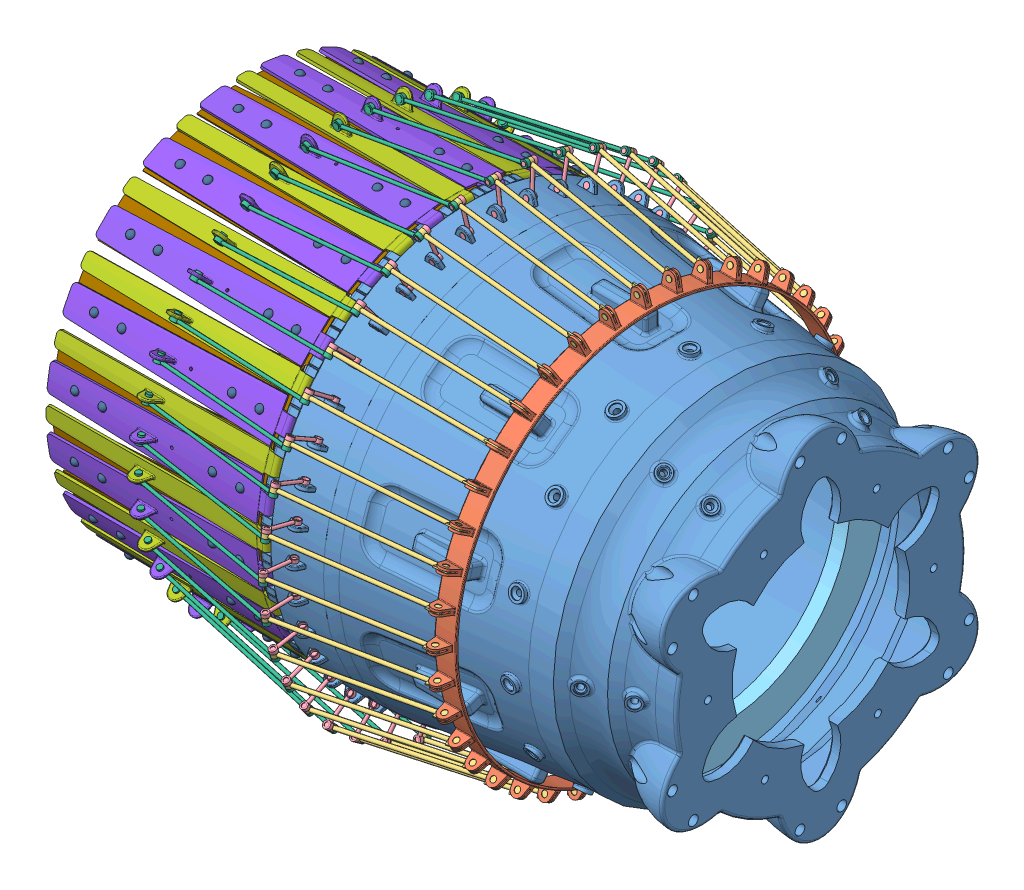
SolidWorks assembly Exhaust Assembly, configuration OPEN . Lengths in mm.
Overall size (418.47 373.17 373.17).
263 component instances, 10 part files, 37 mates.
Components (placement in the parent):
- Part1-1: Part1 [Default] at (233.2329 170.9628 321.4261) size (260.63 300.09 300.09)
- Flare Base-1: Flare Base [Default] at (-84.7671 170.9628 321.4261) x (0 -0.156434 -0.987688) z (1 0 0) size (303.2 303.2 15)
- Flare lever 2-1: Flare lever 2 [Default] at (-182.2053 335.9675 321.4261) x (0 0 -1) z (0.985354 -0.170521 0) size (4.1 7 113)
- Flare Lever 3-1: Flare Lever 3 [Default] at (-182.008 318.4395 318.6761) x (0 0 1) z (-0.120444 0.99272 0) size (8.2 5 25)
- Heat Ring-1: Heat Ring [Default] at (-17.9374 170.9628 321.4261) x (0 -0.257651 0.966238) z (-1 0 0) size (230 230 10)
- Flare Lever 3-2: Flare Lever 3 [Default] at (-182.008 316.1937 295.6395) x (0 0.156434 0.987688) z (-0.120444 0.980498 -0.155296) size (8.2 5 25)
- Flare lever 2-2: Flare lever 2 [Default] at (-182.2053 333.936 295.6137) x (0 -0.156434 -0.987688) z (0.985354 -0.168421 0.026675) size (4.1 7 113)
- Flare lever 1-3: Flare lever 1 [Default] at (-237.8374 326.7848 324.1761) x (0 0 1) z (-0.984613 -0.174748 0) size (6.1 6 116)
- Blade 3-4: Blade 3 [Default] at (-266.5909 130.4236 321.4261) x (0.957917 -0.287045 0) z (0 0 1) size (154.82 49.98 15.19)
- Flare lever 1-4: Flare lever 1 [Default] at (-237.8374 325.2965 299.7663) x (0 0.156434 0.987688) z (-0.984613 -0.172596 0.027337) size (6.1 6 116)
- Blade 4-1: Blade 4 [Default] at (-253.5304 173.9713 320.9496) x (0.957917 -0.283511 0.044904) z (0 0.156434 0.987688) size (154.82 50.19 28.4)
- Blade 1-2: Blade 1 [Default] at (-254.9478 304.5579 299.0391) x (0.957809 -0.285754 0.030748) z (0.017578 0.165029 0.986132) size (146.12 48.38 42.15)
- Rivet-1: Rivet [Default] at (-225.6117 310.4186 298.8323) x (0.988427 0.034217 0.147786) z (0.15131 -0.153019 -0.976571) size (5.66 11 5.66)
- Rivet-2: Rivet [Default] at (-245.6106 310.2053 298.866) x (0.133203 0.156461 0.978661) z (0.99103 -0.010266 -0.133245) size (5.66 11 5.66)
- Rivet-3: Rivet [Default] at (-325.6059 309.3518 299.0012) x (0.133203 0.156461 0.978661) z (0.99103 -0.010266 -0.133245) size (5.66 11 5.66)
- Rivet-4: Rivet [Default] at (-345.6047 309.1385 299.035) x (0.241866 0.15437 0.957951) z (0.97025 -0.027487 -0.240541) size (5.66 11 5.66)
- Rivet-5: Rivet [Default] at (-345.6047 309.2949 342.8295) x (0.241866 -0.149209 0.958769) z (0.97025 0.04819 -0.237263) size (5.66 11 5.66)
- Rivet-6: Rivet [Default] at (-345.6047 295.9104 384.5289) x (0.241866 -0.438182 0.865735) z (0.97025 0.119149 -0.210759) size (5.66 11 5.66)
- Rivet-7: Rivet [Default] at (-345.6047 270.2952 420.0514) x (0.241866 -0.684263 0.687957) z (0.97025 0.178446 -0.163624) size (5.66 11 5.66)
- Rivet-8: Rivet [Default] at (-345.6047 234.9566 445.9198) x (0.241866 -0.863363 0.442838) z (0.97025 0.220275 -0.100473) size (5.66 11 5.66)
- Rivet-9: Rivet [Default] at (-345.6047 193.3539 459.6018) x (0.241866 -0.957951 0.15437) z (0.97025 0.240541 -0.027487) size (5.66 11 5.66)
- Rivet-10: Rivet [Default] at (-345.6047 149.5594 459.7582) x (0.241866 -0.958769 -0.149209) z (0.97025 0.237263 0.04819) size (5.66 11 5.66)
- Rivet-11: Rivet [Default] at (-345.6047 107.86 446.3737) x (0.241866 -0.865735 -0.438182) z (0.97025 0.210759 0.119149) size (5.66 11 5.66)
- Rivet-12: Rivet [Default] at (-345.6047 72.3375 420.7585) x (0.241866 -0.687957 -0.684263) z (0.97025 0.163624 0.178446) size (5.66 11 5.66)
- Rivet-13: Rivet [Default] at (-345.6047 46.4692 385.42) x (0.241866 -0.442838 -0.863363) z (0.97025 0.100473 0.220275) size (5.66 11 5.66)
- Rivet-14: Rivet [Default] at (-345.6047 32.7871 343.8172) x (0.241866 -0.15437 -0.957951) z (0.97025 0.027487 0.240541) size (5.66 11 5.66)
- Rivet-15: Rivet [Default] at (-345.6047 32.6307 300.0227) x (0.241866 0.149209 -0.958769) z (0.97025 -0.04819 0.237263) size (5.66 11 5.66)
- Rivet-16: Rivet [Default] at (-345.6047 46.0152 258.3233) x (0.241866 0.438182 -0.865735) z (0.97025 -0.119149 0.210759) size (5.66 11 5.66)
- Rivet-17: Rivet [Default] at (-345.6047 71.6304 222.8008) x (0.241866 0.684263 -0.687957) z (0.97025 -0.178446 0.163624) size (5.66 11 5.66)
- Rivet-18: Rivet [Default] at (-345.6047 106.969 196.9325) x (0.241866 0.863363 -0.442838) z (0.97025 -0.220275 0.100473) size (5.66 11 5.66)
- Rivet-19: Rivet [Default] at (-345.6047 148.5717 183.2505) x (0.241866 0.957951 -0.15437) z (0.97025 -0.240541 0.027487) size (5.66 11 5.66)
- Rivet-20: Rivet [Default] at (-345.6047 192.3662 183.094) x (0.241866 0.958769 0.149209) z (0.97025 -0.237263 -0.04819) size (5.66 11 5.66)
- Rivet-21: Rivet [Default] at (-345.6047 234.0656 196.4785) x (0.241866 0.865735 0.438182) z (0.97025 -0.210759 -0.119149) size (5.66 11 5.66)
- Rivet-22: Rivet [Default] at (-345.6047 269.5881 222.0937) x (0.241866 0.687957 0.684263) z (0.97025 -0.163624 -0.178446) size (5.66 11 5.66)
- Rivet-23: Rivet [Default] at (-345.6047 295.4564 257.4323) x (0.241866 0.442838 0.863363) z (0.97025 -0.100473 -0.220275) size (5.66 11 5.66)
- Rivet-24: Rivet [Default] at (-325.6059 309.5083 342.8633) x (0.133203 -0.153619 0.979111) z (0.99103 0.031412 -0.129896) size (5.66 11 5.66)
- Rivet-25: Rivet [Default] at (-325.6059 296.1029 384.627) x (0.133203 -0.448662 0.883719) z (0.99103 0.070014 -0.113832) size (5.66 11 5.66)
- Rivet-26: Rivet [Default] at (-325.6059 270.4479 420.2042) x (0.133203 -0.699787 0.701822) z (0.99103 0.101764 -0.086625) size (5.66 11 5.66)
- Rivet-27: Rivet [Default] at (-325.6059 235.0547 446.1122) x (0.133203 -0.882412 0.451226) z (0.99103 0.123552 -0.050939) size (5.66 11 5.66)
- Rivet-28: Rivet [Default] at (-325.6059 193.3877 459.8151) x (0.133203 -0.978661 0.156461) z (0.99103 0.133245 -0.010266) size (5.66 11 5.66)
- Rivet-29: Rivet [Default] at (-325.6059 149.5256 459.9716) x (0.133203 -0.979111 -0.153619) z (0.99103 0.129896 0.031412) size (5.66 11 5.66)
- Rivet-30: Rivet [Default] at (-325.6059 107.7619 446.5662) x (0.133203 -0.883719 -0.448662) z (0.99103 0.113832 0.070014) size (5.66 11 5.66)
- Rivet-31: Rivet [Default] at (-325.6059 72.1847 420.9113) x (0.133203 -0.701822 -0.699787) z (0.99103 0.086625 0.101764) size (5.66 11 5.66)
- Rivet-32: Rivet [Default] at (-325.6059 46.2767 385.518) x (0.133203 -0.451226 -0.882412) z (0.99103 0.050939 0.123552) size (5.66 11 5.66)
- Rivet-33: Rivet [Default] at (-325.6059 32.5738 343.851) x (0.133203 -0.156461 -0.978661) z (0.99103 0.010266 0.133245) size (5.66 11 5.66)
- Rivet-34: Rivet [Default] at (-325.6059 32.4173 299.9889) x (0.133203 0.153619 -0.979111) z (0.99103 -0.031412 0.129896) size (5.66 11 5.66)
- Rivet-35: Rivet [Default] at (-325.6059 45.8227 258.2252) x (0.133203 0.448662 -0.883719) z (0.99103 -0.070014 0.113832) size (5.66 11 5.66)
- Rivet-36: Rivet [Default] at (-325.6059 71.4776 222.6481) x (0.133203 0.699787 -0.701822) z (0.99103 -0.101764 0.086625) size (5.66 11 5.66)
- Rivet-37: Rivet [Default] at (-325.6059 106.8709 196.74) x (0.133203 0.882412 -0.451226) z (0.99103 -0.123552 0.050939) size (5.66 11 5.66)
- Rivet-38: Rivet [Default] at (-325.6059 148.5379 183.0371) x (0.133203 0.978661 -0.156461) z (0.99103 -0.133245 0.010266) size (5.66 11 5.66)
- Rivet-39: Rivet [Default] at (-325.6059 192.4 182.8807) x (0.133203 0.979111 0.153619) z (0.99103 -0.129896 -0.031412) size (5.66 11 5.66)
- Rivet-40: Rivet [Default] at (-325.6059 234.1637 196.286) x (0.133203 0.883719 0.448662) z (0.99103 -0.113832 -0.070014) size (5.66 11 5.66)
- Rivet-41: Rivet [Default] at (-325.6059 269.7408 221.941) x (0.133203 0.701822 0.699787) z (0.99103 -0.086625 -0.101764) size (5.66 11 5.66)
- Rivet-42: Rivet [Default] at (-325.6059 295.6489 257.3342) x (0.133203 0.451226 0.882412) z (0.99103 -0.050939 -0.123552) size (5.66 11 5.66)
- Rivet-43: Rivet [Default] at (-245.6106 310.3617 342.9985) x (0.133203 -0.153619 0.979111) z (0.99103 0.031412 -0.129896) size (5.66 11 5.66)
- Rivet-44: Rivet [Default] at (-245.6106 296.8728 385.0193) x (0.133203 -0.448662 0.883719) z (0.99103 0.070014 -0.113832) size (5.66 11 5.66)
- Rivet-45: Rivet [Default] at (-245.6106 271.0589 420.8152) x (0.133203 -0.699787 0.701822) z (0.99103 0.101764 -0.086625) size (5.66 11 5.66)
- Rivet-46: Rivet [Default] at (-245.6106 235.447 446.8821) x (0.133203 -0.882412 0.451226) z (0.99103 0.123552 -0.050939) size (5.66 11 5.66)
- Rivet-47: Rivet [Default] at (-245.6106 193.5229 460.6686) x (0.133203 -0.978661 0.156461) z (0.99103 0.133245 -0.010266) size (5.66 11 5.66)
- Rivet-48: Rivet [Default] at (-245.6106 149.3904 460.825) x (0.133203 -0.979111 -0.153619) z (0.99103 0.129896 0.031412) size (5.66 11 5.66)
- Rivet-49: Rivet [Default] at (-245.6106 107.3696 447.3361) x (0.133203 -0.883719 -0.448662) z (0.99103 0.113832 0.070014) size (5.66 11 5.66)
- Rivet-50: Rivet [Default] at (-245.6106 71.5738 421.5223) x (0.133203 -0.701822 -0.699787) z (0.99103 0.086625 0.101764) size (5.66 11 5.66)
- Rivet-51: Rivet [Default] at (-245.6106 45.5068 385.9103) x (0.133203 -0.451226 -0.882412) z (0.99103 0.050939 0.123552) size (5.66 11 5.66)
- Rivet-52: Rivet [Default] at (-245.6106 31.7203 343.9862) x (0.133203 -0.156461 -0.978661) z (0.99103 0.010266 0.133245) size (5.66 11 5.66)
- Rivet-53: Rivet [Default] at (-245.6106 31.5639 299.8537) x (0.133203 0.153619 -0.979111) z (0.99103 -0.031412 0.129896) size (5.66 11 5.66)
- Rivet-54: Rivet [Default] at (-245.6106 45.0528 257.8329) x (0.133203 0.448662 -0.883719) z (0.99103 -0.070014 0.113832) size (5.66 11 5.66)
- Rivet-55: Rivet [Default] at (-245.6106 70.8666 222.0371) x (0.133203 0.699787 -0.701822) z (0.99103 -0.101764 0.086625) size (5.66 11 5.66)
- Rivet-56: Rivet [Default] at (-245.6106 106.4786 195.9701) x (0.133203 0.882412 -0.451226) z (0.99103 -0.123552 0.050939) size (5.66 11 5.66)
- Rivet-57: Rivet [Default] at (-245.6106 148.4027 182.1837) x (0.133203 0.978661 -0.156461) z (0.99103 -0.133245 0.010266) size (5.66 11 5.66)
- Rivet-58: Rivet [Default] at (-245.6106 192.5352 182.0272) x (0.133203 0.979111 0.153619) z (0.99103 -0.129896 -0.031412) size (5.66 11 5.66)
- Rivet-59: Rivet [Default] at (-245.6106 234.556 195.5161) x (0.133203 0.883719 0.448662) z (0.99103 -0.113832 -0.070014) size (5.66 11 5.66)
- Rivet-60: Rivet [Default] at (-245.6106 270.3518 221.33) x (0.133203 0.701822 0.699787) z (0.99103 -0.086625 -0.101764) size (5.66 11 5.66)
- Rivet-61: Rivet [Default] at (-245.6106 296.4188 256.9419) x (0.133203 0.451226 0.882412) z (0.99103 -0.050939 -0.123552) size (5.66 11 5.66)
- Rivet-62: Rivet [Default] at (-225.6117 310.5751 343.0323) x (0.988427 -0.013126 0.151126) z (0.15131 0.156247 -0.976059) size (5.66 11 5.66)
- Rivet-63: Rivet [Default] at (-225.6117 297.0653 385.1174) x (0.988427 -0.059184 0.139673) z (0.15131 0.450219 -0.880005) size (5.66 11 5.66)
- Rivet-64: Rivet [Default] at (-225.6117 271.2117 420.9679) x (0.988427 -0.099449 0.114548) z (0.15131 0.70012 -0.697809) size (5.66 11 5.66)
- Rivet-65: Rivet [Default] at (-225.6117 235.5451 447.0746) x (0.988427 -0.129979 0.07821) z (0.15131 0.881489 -0.447307) size (5.66 11 5.66)
- Rivet-66: Rivet [Default] at (-225.6117 193.5567 460.8819) x (0.988427 -0.147786 0.034217) z (0.15131 0.976571 -0.153019) size (5.66 11 5.66)
- Rivet-67: Rivet [Default] at (-225.6117 149.3566 461.0384) x (0.988427 -0.151126 -0.013126) z (0.15131 0.976059 0.156247) size (5.66 11 5.66)
- Rivet-68: Rivet [Default] at (-225.6117 107.2715 447.5286) x (0.988427 -0.139673 -0.059184) z (0.15131 0.880005 0.450219) size (5.66 11 5.66)
- Rivet-69: Rivet [Default] at (-225.6117 71.421 421.675) x (0.988427 -0.114548 -0.099449) z (0.15131 0.697809 0.70012) size (5.66 11 5.66)
- Rivet-70: Rivet [Default] at (-225.6117 45.3143 386.0084) x (0.988427 -0.07821 -0.129979) z (0.15131 0.447307 0.881489) size (5.66 11 5.66)
- Rivet-71: Rivet [Default] at (-225.6117 31.507 344.02) x (0.988427 -0.034217 -0.147786) z (0.15131 0.153019 0.976571) size (5.66 11 5.66)
- Rivet-72: Rivet [Default] at (-225.6117 31.3505 299.8199) x (0.988427 0.013126 -0.151126) z (0.15131 -0.156247 0.976059) size (5.66 11 5.66)
- Rivet-73: Rivet [Default] at (-225.6117 44.8603 257.7349) x (0.988427 0.059184 -0.139673) z (0.15131 -0.450219 0.880005) size (5.66 11 5.66)
- Rivet-74: Rivet [Default] at (-225.6117 70.7139 221.8843) x (0.988427 0.099449 -0.114548) z (0.15131 -0.70012 0.697809) size (5.66 11 5.66)
- Rivet-75: Rivet [Default] at (-225.6117 106.3805 195.7776) x (0.988427 0.129979 -0.07821) z (0.15131 -0.881489 0.447307) size (5.66 11 5.66)
- Rivet-76: Rivet [Default] at (-225.6117 148.3689 181.9703) x (0.988427 0.147786 -0.034217) z (0.15131 -0.976571 0.153019) size (5.66 11 5.66)
- Rivet-77: Rivet [Default] at (-225.6117 192.569 181.8139) x (0.988427 0.151126 0.013126) z (0.15131 -0.976059 -0.156247) size (5.66 11 5.66)
- Rivet-78: Rivet [Default] at (-225.6117 234.6541 195.3236) x (0.988427 0.139673 0.059184) z (0.15131 -0.880005 -0.450219) size (5.66 11 5.66)
- Rivet-79: Rivet [Default] at (-225.6117 270.5046 221.1772) x (0.988427 0.114548 0.099449) z (0.15131 -0.697809 -0.70012) size (5.66 11 5.66)
- Rivet-80: Rivet [Default] at (-225.6117 296.6113 256.8439) x (0.988427 0.07821 0.129979) z (0.15131 -0.447307 -0.881489) size (5.66 11 5.66)
- Blade 1-3: Blade 1 [Default] at (-254.9478 304.9373 341.4179) x (0.957809 -0.28127 -0.05906) z (0.017578 -0.14778 0.988864) size (146.12 48.38 42.15)
- Blade 1-4: Blade 1 [Default] at (-254.9478 292.2023 381.8399) x (0.957809 -0.249253 -0.143086) z (0.017578 -0.446123 0.894799) size (146.12 48.38 42.15)
- Blade 1-5: Blade 1 [Default] at (-254.9478 267.5996 416.3481) x (0.957809 -0.192838 -0.213107) z (0.017578 -0.700796 0.713145) size (146.12 48.38 42.15)
- Blade 1-6: Blade 1 [Default] at (-254.9478 233.5373 441.5647) x (0.957809 -0.117546 -0.262267) z (0.017578 -0.886871 0.461683) size (146.12 48.38 42.15)
- Blade 1-7: Blade 1 [Default] at (-254.9478 193.3498 455.0213) x (0.957809 -0.030748 -0.285754) z (0.017578 -0.986132 0.165029) size (146.12 48.38 42.15)
- Blade 1-8: Blade 1 [Default] at (-254.9478 150.971 455.4006) x (0.957809 0.05906 -0.28127) z (0.017578 -0.988864 -0.14778) size (146.12 48.38 42.15)
- Blade 1-9: Blade 1 [Default] at (-254.9478 110.549 442.6656) x (0.957809 0.143086 -0.249253) z (0.017578 -0.894799 -0.446123) size (146.12 48.38 42.15)
- Blade 1-10: Blade 1 [Default] at (-254.9478 76.0408 418.0629) x (0.957809 0.213107 -0.192838) z (0.017578 -0.713145 -0.700796) size (146.12 48.38 42.15)
- Blade 1-11: Blade 1 [Default] at (-254.9478 50.8242 384.0006) x (0.957809 0.262267 -0.117546) z (0.017578 -0.461683 -0.886871) size (146.12 48.38 42.15)
- Blade 1-12: Blade 1 [Default] at (-254.9478 37.3676 343.8132) x (0.957809 0.285754 -0.030748) z (0.017578 -0.165029 -0.986132) size (146.12 48.38 42.15)
- Blade 1-13: Blade 1 [Default] at (-254.9478 36.9883 301.4343) x (0.957809 0.28127 0.05906) z (0.017578 0.14778 -0.988864) size (146.12 48.38 42.15)
- Blade 1-14: Blade 1 [Default] at (-254.9478 49.7233 261.0124) x (0.957809 0.249253 0.143086) z (0.017578 0.446123 -0.894799) size (146.12 48.38 42.15)
- Blade 1-15: Blade 1 [Default] at (-254.9478 74.326 226.5042) x (0.957809 0.192838 0.213107) z (0.017578 0.700796 -0.713145) size (146.12 48.38 42.15)
- Blade 1-16: Blade 1 [Default] at (-254.9478 108.3883 201.2876) x (0.957809 0.117546 0.262267) z (0.017578 0.886871 -0.461683) size (146.12 48.38 42.15)
- Blade 1-17: Blade 1 [Default] at (-254.9478 148.5757 187.831) x (0.957809 0.030748 0.285754) z (0.017578 0.986132 -0.165029) size (146.12 48.38 42.15)
- Blade 1-18: Blade 1 [Default] at (-254.9478 190.9546 187.4516) x (0.957809 -0.05906 0.28127) z (0.017578 0.988864 0.14778) size (146.12 48.38 42.15)
- Blade 1-19: Blade 1 [Default] at (-254.9478 231.3765 200.1866) x (0.957809 -0.143086 0.249253) z (0.017578 0.894799 0.446123) size (146.12 48.38 42.15)
- Blade 1-20: Blade 1 [Default] at (-254.9478 265.8848 224.7894) x (0.957809 -0.213107 0.192838) z (0.017578 0.713145 0.700796) size (146.12 48.38 42.15)
- Blade 1-21: Blade 1 [Default] at (-254.9478 291.1014 258.8516) x (0.957809 -0.262267 0.117546) z (0.017578 0.461683 0.886871) size (146.12 48.38 42.15)
- Blade 4-2: Blade 4 [Default] at (-253.5304 173.9713 321.9026) x (0.957917 -0.283511 -0.044904) z (0 -0.156434 0.987688) size (154.82 50.19 28.4)
- Blade 4-3: Blade 4 [Default] at (-253.5304 173.6768 322.809) x (0.957917 -0.255759 -0.130316) z (0 -0.45399 0.891007) size (154.82 50.19 28.4)
- Blade 4-4: Blade 4 [Default] at (-253.5304 173.1167 323.58) x (0.957917 -0.202972 -0.202972) z (0 -0.707107 0.707107) size (154.82 50.19 28.4)
- Blade 4-5: Blade 4 [Default] at (-253.5304 172.3457 324.1402) x (0.957917 -0.130316 -0.255759) z (0 -0.891007 0.45399) size (154.82 50.19 28.4)
- Blade 4-6: Blade 4 [Default] at (-253.5304 171.4393 324.4347) x (0.957917 -0.044904 -0.283511) z (0 -0.987688 0.156434) size (154.82 50.19 28.4)
- Blade 4-7: Blade 4 [Default] at (-253.5304 170.4863 324.4347) x (0.957917 0.044904 -0.283511) z (0 -0.987688 -0.156434) size (154.82 50.19 28.4)
- Blade 4-8: Blade 4 [Default] at (-253.5304 169.5799 324.1402) x (0.957917 0.130316 -0.255759) z (0 -0.891007 -0.45399) size (154.82 50.19 28.4)
- Blade 4-9: Blade 4 [Default] at (-253.5304 168.8089 323.58) x (0.957917 0.202972 -0.202972) z (0 -0.707107 -0.707107) size (154.82 50.19 28.4)
- Blade 4-10: Blade 4 [Default] at (-253.5304 168.2488 322.809) x (0.957917 0.255759 -0.130316) z (0 -0.45399 -0.891007) size (154.82 50.19 28.4)
- Blade 4-11: Blade 4 [Default] at (-253.5304 167.9543 321.9026) x (0.957917 0.283511 -0.044904) z (0 -0.156434 -0.987688) size (154.82 50.19 28.4)
- Blade 4-12: Blade 4 [Default] at (-253.5304 167.9543 320.9496) x (0.957917 0.283511 0.044904) z (0 0.156434 -0.987688) size (154.82 50.19 28.4)
- Blade 4-13: Blade 4 [Default] at (-253.5304 168.2488 320.0432) x (0.957917 0.255759 0.130316) z (0 0.45399 -0.891007) size (154.82 50.19 28.4)
- Blade 4-14: Blade 4 [Default] at (-253.5304 168.8089 319.2722) x (0.957917 0.202972 0.202972) z (0 0.707107 -0.707107) size (154.82 50.19 28.4)
- Blade 4-15: Blade 4 [Default] at (-253.5304 169.5799 318.7121) x (0.957917 0.130316 0.255759) z (0 0.891007 -0.45399) size (154.82 50.19 28.4)
- Blade 4-16: Blade 4 [Default] at (-253.5304 170.4863 318.4176) x (0.957917 0.044904 0.283511) z (0 0.987688 -0.156434) size (154.82 50.19 28.4)
- Blade 4-17: Blade 4 [Default] at (-253.5304 171.4393 318.4176) x (0.957917 -0.044904 0.283511) z (0 0.987688 0.156434) size (154.82 50.19 28.4)
- Blade 4-18: Blade 4 [Default] at (-253.5304 172.3457 318.7121) x (0.957917 -0.130316 0.255759) z (0 0.891007 0.45399) size (154.82 50.19 28.4)
- Blade 4-19: Blade 4 [Default] at (-253.5304 173.1167 319.2722) x (0.957917 -0.202972 0.202972) z (0 0.707107 0.707107) size (154.82 50.19 28.4)
- Blade 4-20: Blade 4 [Default] at (-253.5304 173.6768 320.0432) x (0.957917 -0.255759 0.130316) z (0 0.45399 0.891007) size (154.82 50.19 28.4)
- Flare lever 1-5: Flare lever 1 [Default] at (-237.8374 324.4361 348.5182) x (0 -0.156434 0.987688) z (-0.984613 -0.172596 -0.027337) size (6.1 6 116)
- Flare lever 1-6: Flare lever 1 [Default] at (-237.8374 308.5527 394.6181) x (0 -0.45399 0.891007) z (-0.984613 -0.155701 -0.079334) size (6.1 6 116)
- Flare lever 1-7: Flare lever 1 [Default] at (-237.8374 279.201 433.5534) x (0 -0.707107 0.707107) z (-0.984613 -0.123565 -0.123565) size (6.1 6 116)
- Flare lever 1-8: Flare lever 1 [Default] at (-237.8374 239.2542 461.513) x (0 -0.891007 0.45399) z (-0.984613 -0.079334 -0.155701) size (6.1 6 116)
- Flare lever 1-9: Flare lever 1 [Default] at (-237.8374 192.6226 475.7598) x (0 -0.987688 0.156434) z (-0.984613 -0.027337 -0.172596) size (6.1 6 116)
- Flare lever 1-10: Flare lever 1 [Default] at (-237.8374 143.8707 474.8995) x (0 -0.987688 -0.156434) z (-0.984613 0.027337 -0.172596) size (6.1 6 116)
- Flare lever 1-11: Flare lever 1 [Default] at (-237.8374 97.7708 459.016) x (0 -0.891007 -0.45399) z (-0.984613 0.079334 -0.155701) size (6.1 6 116)
- Flare lever 1-12: Flare lever 1 [Default] at (-237.8374 58.8355 429.6643) x (0 -0.707107 -0.707107) z (-0.984613 0.123565 -0.123565) size (6.1 6 116)
- Flare lever 1-13: Flare lever 1 [Default] at (-237.8374 30.8759 389.7175) x (0 -0.45399 -0.891007) z (-0.984613 0.155701 -0.079334) size (6.1 6 116)
- Flare lever 1-14: Flare lever 1 [Default] at (-237.8374 16.6291 343.0859) x (0 -0.156434 -0.987688) z (-0.984613 0.172596 -0.027337) size (6.1 6 116)
- Flare lever 1-15: Flare lever 1 [Default] at (-237.8374 17.4895 294.334) x (0 0.156434 -0.987688) z (-0.984613 0.172596 0.027337) size (6.1 6 116)
- Flare lever 1-16: Flare lever 1 [Default] at (-237.8374 33.3729 248.2342) x (0 0.45399 -0.891007) z (-0.984613 0.155701 0.079334) size (6.1 6 116)
- Flare lever 1-17: Flare lever 1 [Default] at (-237.8374 62.7246 209.2988) x (0 0.707107 -0.707107) z (-0.984613 0.123565 0.123565) size (6.1 6 116)
- Flare lever 1-18: Flare lever 1 [Default] at (-237.8374 102.6714 181.3393) x (0 0.891007 -0.45399) z (-0.984613 0.079334 0.155701) size (6.1 6 116)
- Flare lever 1-19: Flare lever 1 [Default] at (-237.8374 149.303 167.0924) x (0 0.987688 -0.156434) z (-0.984613 0.027337 0.172596) size (6.1 6 116)
- Flare lever 1-20: Flare lever 1 [Default] at (-237.8374 198.0549 167.9528) x (0 0.987688 0.156434) z (-0.984613 -0.027337 0.172596) size (6.1 6 116)
- Flare lever 1-21: Flare lever 1 [Default] at (-237.8374 244.1548 183.8362) x (0 0.891007 0.45399) z (-0.984613 -0.079334 0.155701) size (6.1 6 116)
- Flare lever 1-22: Flare lever 1 [Default] at (-237.8374 283.0901 213.1879) x (0 0.707107 0.707107) z (-0.984613 -0.123565 0.123565) size (6.1 6 116)
- Flare lever 1-23: Flare lever 1 [Default] at (-237.8374 311.0497 253.1347) x (0 0.45399 0.891007) z (-0.984613 -0.155701 0.079334) size (6.1 6 116)
- Blade 3-5: Blade 3 [Default] at (-266.5909 132.4077 308.8988) x (0.957917 -0.272996 -0.088702) z (0 -0.309017 0.951057) size (154.82 49.98 15.19)
- Blade 3-6: Blade 3 [Default] at (-266.5909 138.1659 297.5978) x (0.957917 -0.232224 -0.168721) z (0 -0.587785 0.809017) size (154.82 49.98 15.19)
- Blade 3-7: Blade 3 [Default] at (-266.5909 147.1345 288.6292) x (0.957917 -0.168721 -0.232224) z (0 -0.809017 0.587785) size (154.82 49.98 15.19)
- Blade 3-8: Blade 3 [Default] at (-266.5909 158.4355 282.8711) x (0.957917 -0.088702 -0.272996) z (0 -0.951057 0.309017) size (154.82 49.98 15.19)
- Blade 3-9: Blade 3 [Default] at (-266.5909 170.9628 280.8869) x (0.957917 0 -0.287045) z (0 -1 0) size (154.82 49.98 15.19)
- Blade 3-10: Blade 3 [Default] at (-266.5909 183.4901 282.8711) x (0.957917 0.088702 -0.272996) z (0 -0.951057 -0.309017) size (154.82 49.98 15.19)
- Blade 3-11: Blade 3 [Default] at (-266.5909 194.7911 288.6292) x (0.957917 0.168721 -0.232224) z (0 -0.809017 -0.587785) size (154.82 49.98 15.19)
- Blade 3-12: Blade 3 [Default] at (-266.5909 203.7597 297.5978) x (0.957917 0.232224 -0.168721) z (0 -0.587785 -0.809017) size (154.82 49.98 15.19)
- Blade 3-13: Blade 3 [Default] at (-266.5909 209.5178 308.8988) x (0.957917 0.272996 -0.088702) z (0 -0.309017 -0.951057) size (154.82 49.98 15.19)
- Blade 3-14: Blade 3 [Default] at (-266.5909 211.502 321.4261) x (0.957917 0.287045 0) z (0 0 -1) size (154.82 49.98 15.19)
- Blade 3-15: Blade 3 [Default] at (-266.5909 209.5178 333.9534) x (0.957917 0.272996 0.088702) z (0 0.309017 -0.951057) size (154.82 49.98 15.19)
- Blade 3-16: Blade 3 [Default] at (-266.5909 203.7597 345.2545) x (0.957917 0.232224 0.168721) z (0 0.587785 -0.809017) size (154.82 49.98 15.19)
- Blade 3-17: Blade 3 [Default] at (-266.5909 194.7911 354.223) x (0.957917 0.168721 0.232224) z (0 0.809017 -0.587785) size (154.82 49.98 15.19)
- Blade 3-18: Blade 3 [Default] at (-266.5909 183.4901 359.9812) x (0.957917 0.088702 0.272996) z (0 0.951057 -0.309017) size (154.82 49.98 15.19)
- Blade 3-19: Blade 3 [Default] at (-266.5909 170.9628 361.9653) x (0.957917 0 0.287045) z (0 1 0) size (154.82 49.98 15.19)
- Blade 3-20: Blade 3 [Default] at (-266.5909 158.4355 359.9812) x (0.957917 -0.088702 0.272996) z (0 0.951057 0.309017) size (154.82 49.98 15.19)
- Blade 3-21: Blade 3 [Default] at (-266.5909 147.1345 354.223) x (0.957917 -0.168721 0.232224) z (0 0.809017 0.587785) size (154.82 49.98 15.19)
- Blade 3-22: Blade 3 [Default] at (-266.5909 138.1659 345.2545) x (0.957917 -0.232224 0.168721) z (0 0.587785 0.809017) size (154.82 49.98 15.19)
- Blade 3-23: Blade 3 [Default] at (-266.5909 132.4077 333.9534) x (0.957917 -0.272996 0.088702) z (0 0.309017 0.951057) size (154.82 49.98 15.19)
- Flare lever 1-24: Flare lever 1 [Default] at (-237.8374 318.3085 372.1932) x (0 -0.309017 0.951057) z (-0.984613 -0.166195 -0.054) size (6.1 6 116)
- Flare lever 1-25: Flare lever 1 [Default] at (-237.8374 295.409 415.2408) x (0 -0.587785 0.809017) z (-0.984613 -0.141374 -0.102714) size (6.1 6 116)
- Flare lever 1-26: Flare lever 1 [Default] at (-237.8374 260.3278 449.1051) x (0 -0.809017 0.587785) z (-0.984613 -0.102714 -0.141374) size (6.1 6 116)
- Flare lever 1-27: Flare lever 1 [Default] at (-237.8374 216.499 470.4714) x (0 -0.951057 0.309017) z (-0.984613 -0.054 -0.166195) size (6.1 6 116)
- Flare lever 1-28: Flare lever 1 [Default] at (-237.8374 168.2128 477.2481) x (0 -1 0) z (-0.984613 0 -0.174748) size (6.1 6 116)
- Flare lever 1-29: Flare lever 1 [Default] at (-237.8374 120.1958 468.7718) x (0 -0.951057 -0.309017) z (-0.984613 0.054 -0.166195) size (6.1 6 116)
- Flare lever 1-30: Flare lever 1 [Default] at (-237.8374 77.1481 445.8723) x (0 -0.809017 -0.587785) z (-0.984613 0.102714 -0.141374) size (6.1 6 116)
- Flare lever 1-31: Flare lever 1 [Default] at (-237.8374 43.2838 410.7912) x (0 -0.587785 -0.809017) z (-0.984613 0.141374 -0.102714) size (6.1 6 116)
- Flare lever 1-32: Flare lever 1 [Default] at (-237.8374 21.9175 366.9623) x (0 -0.309017 -0.951057) z (-0.984613 0.166195 -0.054) size (6.1 6 116)
- Flare lever 1-33: Flare lever 1 [Default] at (-237.8374 15.1408 318.6761) x (0 0 -1) z (-0.984613 0.174748 0) size (6.1 6 116)
- Flare lever 1-34: Flare lever 1 [Default] at (-237.8374 23.6171 270.6591) x (0 0.309017 -0.951057) z (-0.984613 0.166195 0.054) size (6.1 6 116)
- Flare lever 1-35: Flare lever 1 [Default] at (-237.8374 46.5166 227.6115) x (0 0.587785 -0.809017) z (-0.984613 0.141374 0.102714) size (6.1 6 116)
- Flare lever 1-36: Flare lever 1 [Default] at (-237.8374 81.5977 193.7471) x (0 0.809017 -0.587785) z (-0.984613 0.102714 0.141374) size (6.1 6 116)
- Flare lever 1-37: Flare lever 1 [Default] at (-237.8374 125.4266 172.3808) x (0 0.951057 -0.309017) z (-0.984613 0.054 0.166195) size (6.1 6 116)
- Flare lever 1-38: Flare lever 1 [Default] at (-237.8374 173.7128 165.6042) x (0 1 0) z (-0.984613 0 0.174748) size (6.1 6 116)
- Flare lever 1-39: Flare lever 1 [Default] at (-237.8374 221.7298 174.0804) x (0 0.951057 0.309017) z (-0.984613 -0.054 0.166195) size (6.1 6 116)
- Flare lever 1-40: Flare lever 1 [Default] at (-237.8374 264.7774 196.9799) x (0 0.809017 0.587785) z (-0.984613 -0.102714 0.141374) size (6.1 6 116)
- Flare lever 1-41: Flare lever 1 [Default] at (-237.8374 298.6418 232.0611) x (0 0.587785 0.809017) z (-0.984613 -0.141374 0.102714) size (6.1 6 116)
- Flare lever 1-42: Flare lever 1 [Default] at (-237.8374 320.0081 275.8899) x (0 0.309017 0.951057) z (-0.984613 -0.166195 0.054) size (6.1 6 116)
- Flare lever 2-3: Flare lever 2 [Default] at (-182.2053 333.936 347.2385) x (0 0.156434 -0.987688) z (0.985354 -0.168421 -0.026675) size (4.1 7 113)
- Flare lever 2-4: Flare lever 2 [Default] at (-182.2053 317.983 396.3367) x (0 0.45399 -0.891007) z (0.985354 -0.151935 -0.077415) size (4.1 7 113)
- Flare lever 2-5: Flare lever 2 [Default] at (-182.2053 287.6387 438.102) x (0 0.707107 -0.707107) z (0.985354 -0.120576 -0.120576) size (4.1 7 113)
- Flare lever 2-6: Flare lever 2 [Default] at (-182.2053 245.8733 468.4463) x (0 0.891007 -0.45399) z (0.985354 -0.077415 -0.151935) size (4.1 7 113)
- Flare lever 2-7: Flare lever 2 [Default] at (-182.2053 196.7752 484.3993) x (0 0.987688 -0.156434) z (0.985354 -0.026675 -0.168421) size (4.1 7 113)
- Flare lever 2-8: Flare lever 2 [Default] at (-182.2053 145.1504 484.3993) x (0 0.987688 0.156434) z (0.985354 0.026675 -0.168421) size (4.1 7 113)
- Flare lever 2-9: Flare lever 2 [Default] at (-182.2053 96.0522 468.4463) x (0 0.891007 0.45399) z (0.985354 0.077415 -0.151935) size (4.1 7 113)
- Flare lever 2-10: Flare lever 2 [Default] at (-182.2053 54.2869 438.102) x (0 0.707107 0.707107) z (0.985354 0.120576 -0.120576) size (4.1 7 113)
- Flare lever 2-11: Flare lever 2 [Default] at (-182.2053 23.9426 396.3367) x (0 0.45399 0.891007) z (0.985354 0.151935 -0.077415) size (4.1 7 113)
- Flare lever 2-12: Flare lever 2 [Default] at (-182.2053 7.9896 347.2385) x (0 0.156434 0.987688) z (0.985354 0.168421 -0.026675) size (4.1 7 113)
- Flare lever 2-13: Flare lever 2 [Default] at (-182.2053 7.9896 295.6137) x (0 -0.156434 0.987688) z (0.985354 0.168421 0.026675) size (4.1 7 113)
- Flare lever 2-14: Flare lever 2 [Default] at (-182.2053 23.9426 246.5156) x (0 -0.45399 0.891007) z (0.985354 0.151935 0.077415) size (4.1 7 113)
- Flare lever 2-15: Flare lever 2 [Default] at (-182.2053 54.2869 204.7502) x (0 -0.707107 0.707107) z (0.985354 0.120576 0.120576) size (4.1 7 113)
- Flare lever 2-16: Flare lever 2 [Default] at (-182.2053 96.0522 174.4059) x (0 -0.891007 0.45399) z (0.985354 0.077415 0.151935) size (4.1 7 113)
- Flare lever 2-17: Flare lever 2 [Default] at (-182.2053 145.1504 158.4529) x (0 -0.987688 0.156434) z (0.985354 0.026675 0.168421) size (4.1 7 113)
- Flare lever 2-18: Flare lever 2 [Default] at (-182.2053 196.7752 158.4529) x (0 -0.987688 -0.156434) z (0.985354 -0.026675 0.168421) size (4.1 7 113)
- Flare lever 2-19: Flare lever 2 [Default] at (-182.2053 245.8733 174.4059) x (0 -0.891007 -0.45399) z (0.985354 -0.077415 0.151935) size (4.1 7 113)
- Flare lever 2-20: Flare lever 2 [Default] at (-182.2053 287.6387 204.7502) x (0 -0.707107 -0.707107) z (0.985354 -0.120576 0.120576) size (4.1 7 113)
- Flare lever 2-21: Flare lever 2 [Default] at (-182.2053 317.983 246.5156) x (0 -0.45399 -0.891007) z (0.985354 -0.151935 0.077415) size (4.1 7 113)
- Flare Lever 3-4: Flare Lever 3 [Default] at (-182.008 317.054 341.7804) x (0 -0.156434 0.987688) z (-0.120444 0.980498 0.155296) size (8.2 5 25)
- Flare Lever 3-5: Flare Lever 3 [Default] at (-182.008 303.614 385.9289) x (0 -0.45399 0.891007) z (-0.120444 0.88452 0.450685) size (8.2 5 25)
- Flare Lever 3-6: Flare Lever 3 [Default] at (-182.008 277.1891 423.7634) x (0 -0.707107 0.707107) z (-0.120444 0.701959 0.701959) size (8.2 5 25)
- Flare Lever 3-7: Flare Lever 3 [Default] at (-182.008 240.3661 451.5804) x (0 -0.891007 0.45399) z (-0.120444 0.450685 0.88452) size (8.2 5 25)
- Flare Lever 3-8: Flare Lever 3 [Default] at (-182.008 196.7494 466.657) x (0 -0.987688 0.156434) z (-0.120444 0.155296 0.980498) size (8.2 5 25)
- Flare Lever 3-9: Flare Lever 3 [Default] at (-182.008 150.6085 467.5174) x (0 -0.987688 -0.156434) z (-0.120444 -0.155296 0.980498) size (8.2 5 25)
- Flare Lever 3-10: Flare Lever 3 [Default] at (-182.008 106.46 454.0773) x (0 -0.891007 -0.45399) z (-0.120444 -0.450685 0.88452) size (8.2 5 25)
- Flare Lever 3-11: Flare Lever 3 [Default] at (-182.008 68.6255 427.6525) x (0 -0.707107 -0.707107) z (-0.120444 -0.701959 0.701959) size (8.2 5 25)
- Flare Lever 3-12: Flare Lever 3 [Default] at (-182.008 40.8085 390.8294) x (0 -0.45399 -0.891007) z (-0.120444 -0.88452 0.450685) size (8.2 5 25)
- Flare Lever 3-13: Flare Lever 3 [Default] at (-182.008 25.7319 347.2127) x (0 -0.156434 -0.987688) z (-0.120444 -0.980498 0.155296) size (8.2 5 25)
- Flare Lever 3-14: Flare Lever 3 [Default] at (-182.008 24.8715 301.0718) x (0 0.156434 -0.987688) z (-0.120444 -0.980498 -0.155296) size (8.2 5 25)
- Flare Lever 3-15: Flare Lever 3 [Default] at (-182.008 38.3116 256.9233) x (0 0.45399 -0.891007) z (-0.120444 -0.88452 -0.450685) size (8.2 5 25)
- Flare Lever 3-16: Flare Lever 3 [Default] at (-182.008 64.7364 219.0889) x (0 0.707107 -0.707107) z (-0.120444 -0.701959 -0.701959) size (8.2 5 25)
- Flare Lever 3-17: Flare Lever 3 [Default] at (-182.008 101.5595 191.2719) x (0 0.891007 -0.45399) z (-0.120444 -0.450685 -0.88452) size (8.2 5 25)
- Flare Lever 3-18: Flare Lever 3 [Default] at (-182.008 145.1762 176.1953) x (0 0.987688 -0.156434) z (-0.120444 -0.155296 -0.980498) size (8.2 5 25)
- Flare Lever 3-19: Flare Lever 3 [Default] at (-182.008 191.3171 175.3349) x (0 0.987688 0.156434) z (-0.120444 0.155296 -0.980498) size (8.2 5 25)
- Flare Lever 3-20: Flare Lever 3 [Default] at (-182.008 235.4656 188.7749) x (0 0.891007 0.45399) z (-0.120444 0.450685 -0.88452) size (8.2 5 25)
- Flare Lever 3-21: Flare Lever 3 [Default] at (-182.008 273.3001 215.1998) x (0 0.707107 0.707107) z (-0.120444 0.701959 -0.701959) size (8.2 5 25)
- Flare Lever 3-22: Flare Lever 3 [Default] at (-182.008 301.1171 252.0228) x (0 0.45399 0.891007) z (-0.120444 0.88452 -0.450685) size (8.2 5 25)
- Flare Lever 3-23: Flare Lever 3 [Default] at (-182.008 312.0713 364.3835) x (0 -0.309017 0.951057) z (-0.120444 0.944133 0.306767) size (8.2 5 25)
- Flare Lever 3-24: Flare Lever 3 [Default] at (-182.008 291.8904 405.886) x (0 -0.587785 0.809017) z (-0.120444 0.803127 0.583506) size (8.2 5 25)
- Flare Lever 3-25: Flare Lever 3 [Default] at (-182.008 259.8722 439.1209) x (0 -0.809017 0.587785) z (-0.120444 0.583506 0.803127) size (8.2 5 25)
- Flare Lever 3-26: Flare Lever 3 [Default] at (-182.008 219.151 460.835) x (0 -0.951057 0.309017) z (-0.120444 0.306767 0.944133) size (8.2 5 25)
- Flare Lever 3-27: Flare Lever 3 [Default] at (-182.008 173.7128 468.9029) x (0 -1 0) z (-0.120444 0 0.99272) size (8.2 5 25)
- Flare Lever 3-28: Flare Lever 3 [Default] at (-182.008 128.0054 462.5346) x (0 -0.951057 -0.309017) z (-0.120444 -0.306767 0.944133) size (8.2 5 25)
- Flare Lever 3-29: Flare Lever 3 [Default] at (-182.008 86.5029 442.3537) x (0 -0.809017 -0.587785) z (-0.120444 -0.583506 0.803127) size (8.2 5 25)
- Flare Lever 3-30: Flare Lever 3 [Default] at (-182.008 53.268 410.3356) x (0 -0.587785 -0.809017) z (-0.120444 -0.803127 0.583506) size (8.2 5 25)
- Flare Lever 3-31: Flare Lever 3 [Default] at (-182.008 31.5539 369.6143) x (0 -0.309017 -0.951057) z (-0.120444 -0.944133 0.306767) size (8.2 5 25)
- Flare Lever 3-32: Flare Lever 3 [Default] at (-182.008 23.4861 324.1761) x (0 0 -1) z (-0.120444 -0.99272 0) size (8.2 5 25)
- Flare Lever 3-33: Flare Lever 3 [Default] at (-182.008 29.8543 278.4687) x (0 0.309017 -0.951057) z (-0.120444 -0.944133 -0.306767) size (8.2 5 25)
- Flare Lever 3-34: Flare Lever 3 [Default] at (-182.008 50.0352 236.9663) x (0 0.587785 -0.809017) z (-0.120444 -0.803127 -0.583506) size (8.2 5 25)
- Flare Lever 3-35: Flare Lever 3 [Default] at (-182.008 82.0533 203.7313) x (0 0.809017 -0.587785) z (-0.120444 -0.583506 -0.803127) size (8.2 5 25)
- Flare Lever 3-36: Flare Lever 3 [Default] at (-182.008 122.7746 182.0172) x (0 0.951057 -0.309017) z (-0.120444 -0.306767 -0.944133) size (8.2 5 25)
- Flare Lever 3-37: Flare Lever 3 [Default] at (-182.008 168.2128 173.9494) x (0 1 0) z (-0.120444 0 -0.99272) size (8.2 5 25)
- Flare Lever 3-38: Flare Lever 3 [Default] at (-182.008 213.9202 180.3176) x (0 0.951057 0.309017) z (-0.120444 0.306767 -0.944133) size (8.2 5 25)
- Flare Lever 3-39: Flare Lever 3 [Default] at (-182.008 255.4227 200.4985) x (0 0.809017 0.587785) z (-0.120444 0.583506 -0.803127) size (8.2 5 25)
- Flare Lever 3-40: Flare Lever 3 [Default] at (-182.008 288.6576 232.5167) x (0 0.587785 0.809017) z (-0.120444 0.803127 -0.583506) size (8.2 5 25)
- Flare Lever 3-41: Flare Lever 3 [Default] at (-182.008 310.3717 273.2379) x (0 0.309017 0.951057) z (-0.120444 0.944133 -0.306767) size (8.2 5 25)
- Flare lever 2-22: Flare lever 2 [Default] at (-182.2053 327.8916 372.4154) x (0 0.309017 -0.951057) z (0.985354 -0.162175 -0.052694) size (4.1 7 113)
- Flare lever 2-23: Flare lever 2 [Default] at (-182.2053 304.4544 418.4134) x (0 0.587785 -0.809017) z (0.985354 -0.137954 -0.100229) size (4.1 7 113)
- Flare lever 2-24: Flare lever 2 [Default] at (-182.2053 267.9501 454.9177) x (0 0.809017 -0.587785) z (0.985354 -0.100229 -0.137954) size (4.1 7 113)
- Flare lever 2-25: Flare lever 2 [Default] at (-182.2053 221.952 478.3549) x (0 0.951057 -0.309017) z (0.985354 -0.052694 -0.162175) size (4.1 7 113)
- Flare lever 2-26: Flare lever 2 [Default] at (-182.2053 170.9628 486.4308) x (0 1 0) z (0.985354 0 -0.170521) size (4.1 7 113)
- Flare lever 2-27: Flare lever 2 [Default] at (-182.2053 119.9735 478.3549) x (0 0.951057 0.309017) z (0.985354 0.052694 -0.162175) size (4.1 7 113)
- Flare lever 2-28: Flare lever 2 [Default] at (-182.2053 73.9755 454.9177) x (0 0.809017 0.587785) z (0.985354 0.100229 -0.137954) size (4.1 7 113)
- Flare lever 2-29: Flare lever 2 [Default] at (-182.2053 37.4712 418.4134) x (0 0.587785 0.809017) z (0.985354 0.137954 -0.100229) size (4.1 7 113)
- Flare lever 2-30: Flare lever 2 [Default] at (-182.2053 14.034 372.4154) x (0 0.309017 0.951057) z (0.985354 0.162175 -0.052694) size (4.1 7 113)
- Flare lever 2-31: Flare lever 2 [Default] at (-182.2053 5.9581 321.4261) x (0 0 1) z (0.985354 0.170521 0) size (4.1 7 113)
- Flare lever 2-32: Flare lever 2 [Default] at (-182.2053 14.034 270.4369) x (0 -0.309017 0.951057) z (0.985354 0.162175 0.052694) size (4.1 7 113)
- Flare lever 2-33: Flare lever 2 [Default] at (-182.2053 37.4712 224.4388) x (0 -0.587785 0.809017) z (0.985354 0.137954 0.100229) size (4.1 7 113)
- Flare lever 2-34: Flare lever 2 [Default] at (-182.2053 73.9755 187.9345) x (0 -0.809017 0.587785) z (0.985354 0.100229 0.137954) size (4.1 7 113)
- Flare lever 2-35: Flare lever 2 [Default] at (-182.2053 119.9735 164.4974) x (0 -0.951057 0.309017) z (0.985354 0.052694 0.162175) size (4.1 7 113)
- Flare lever 2-36: Flare lever 2 [Default] at (-182.2053 170.9628 156.4215) x (0 -1 0) z (0.985354 0 0.170521) size (4.1 7 113)
- Flare lever 2-37: Flare lever 2 [Default] at (-182.2053 221.952 164.4974) x (0 -0.951057 -0.309017) z (0.985354 -0.052694 0.162175) size (4.1 7 113)
- Flare lever 2-38: Flare lever 2 [Default] at (-182.2053 267.9501 187.9345) x (0 -0.809017 -0.587785) z (0.985354 -0.100229 0.137954) size (4.1 7 113)
- Flare lever 2-39: Flare lever 2 [Default] at (-182.2053 304.4544 224.4388) x (0 -0.587785 -0.809017) z (0.985354 -0.137954 0.100229) size (4.1 7 113)
- Flare lever 2-40: Flare lever 2 [Default] at (-182.2053 327.8916 270.4369) x (0 -0.309017 -0.951057) z (0.985354 -0.162175 0.052694) size (4.1 7 113)
Mates (geometry in assembly coordinates):
- Concentric1: concentric anti-aligned: cylinder of Part1-1 through (233.2329 170.9628 321.4261) axis (1 0 0) radius 143.2935; cylinder of Flare Base-1 through (-77.2261 170.9628 321.4261) axis (-1 0 0) radius 140
- Distance1: distance = 0 mm aligned: plane of Part1-1 through (-69.7671 20.9182 324.4261) normal (1 0 0); plane of Flare Base-1 through (-69.7671 170.9628 321.4261) normal (1 0 0)
- Width2: width anti-aligned: plane of Flare lever 2-1 through (-82.2311 321.0176 320.9261) normal (0 0 -1); plane of Flare lever 2-1 through (-82.2311 321.0176 321.9261) normal (0 0 1); plane of Flare Base-1 through (-86.2021 318.0628 320.9261) normal (0 0 1); plane of Flare Base-1 through (-86.2021 318.0628 321.9261) normal (0 0 -1)
- Concentric3: concentric anti-aligned: cylinder of Flare Base-1 through (-86.2021 318.0628 319.4261) axis (0 0 1) radius 2; cylinder of Flare lever 2-1 through (-86.2021 318.0628 323.8261) axis (0 0 -1) radius 2
- Concentric4: concentric anti-aligned: circle of Flare lever 2-1; cylinder of Flare Lever 3-1 through (-192.0685 333.5971 325.6261) axis (0 0 -1) radius 1.5
- Coincident3: coincident anti-aligned: plane of Flare lever 2-1 through (-190.5843 333.3793 319.9261) normal (0 0 -1); plane of Flare Lever 3-1 through (-190.7808 331.4542 319.9261) normal (0 0 1)
- Concentric5: concentric anti-aligned: cylinder of Part1-1 through (-181.7671 316.4541 319.9261) axis (0 0 1) radius 2; cylinder of Flare Lever 3-1 through (-181.7671 316.4541 323.1261) axis (0 0 -1) radius 2
- Concentric6: concentric aligned: cone of Part1-1 through (-32.2671 170.9628 321.4261) axis (1 0 0); cylinder of Heat Ring-1 through (-27.9374 170.9628 321.4261) axis (1 0 0) radius 115
- Coincident5: coincident anti-aligned: plane of Flare Lever 3-2 through (-190.7808 329.2436 294.8382) normal (0 0.156434 0.987688); plane of Flare lever 2-2 through (-190.5843 331.145 294.537) normal (0 -0.156434 -0.987688)
- Concentric9: concentric anti-aligned: cylinder of Flare Lever 3-2 through (-192.0685 332.2518 300.1328) axis (0 -0.156434 -0.987688) radius 1.5; circle of Flare lever 2-2
- Width3: width aligned: plane of Flare lever 2-2 through (-82.2311 319.2484 298.4462) normal (0 0.156434 0.987688); plane of Flare lever 2-2 through (-82.2311 319.0919 297.4585) normal (0 -0.156434 -0.987688); plane of Flare Base-1 through (-86.2021 316.1735 297.9208) normal (0 0.156434 0.987688); plane of Flare Base-1 through (-86.2021 316.33 298.9085) normal (0 -0.156434 -0.987688)
- Concentric10: concentric anti-aligned: cylinder of Flare Base-1 through (-86.2021 315.9389 296.4392) axis (0 0.156434 0.987688) radius 2; cylinder of Flare lever 2-2 through (-86.2021 316.6272 300.7851) axis (0 -0.156434 -0.987688) radius 2
- Concentric11: concentric anti-aligned: cylinder of Part1-1 through (-181.7671 314.4282 297.1847) axis (0 0.156434 0.987688) radius 2; cylinder of Flare Lever 3-2 through (-181.7671 314.9288 300.3453) axis (0 -0.156434 -0.987688) radius 2
- Concentric25: concentric aligned: cylinder of Flare Lever 3-1 through (-192.0685 333.5971 325.6261) axis (0 0 -1) radius 1.5; cylinder of Flare lever 1-3 through (-192.0685 333.5971 322.4137) axis (0 0 -1) radius 1.5
- Coincident16: coincident anti-aligned: plane of Flare lever 2-1 through (-190.5843 333.3793 322.9261) normal (0 0 1); plane of Flare lever 1-3 through (-193.3121 332.7584 322.9261) normal (0 0 -1)
- Concentric26: concentric aligned: cylinder of Flare lever 1-3 through (-283.6842 271.8168 319.6261) axis (0 0 1) radius 2; circle of Blade 3-4
- Coincident18: coincident anti-aligned: plane of Flare lever 1-3 through (-281.1969 273.4941 322.9261) normal (0 0 -1); plane of Blade 3-4 through (-284.1076 272.5145 322.9261) normal (0 0 1)
- Concentric29: concentric aligned: cylinder of Part1-1 through (-206.4008 311.2563 332.2761) axis (0 0 -1) radius 3; cylinder of Blade 3-4 through (-206.4008 311.2563 327.7706) axis (0 0 -1) radius 2.76
- Concentric30: concentric aligned: cylinder of Flare Lever 3-2 through (-192.0685 332.2518 300.1328) axis (0 -0.156434 -0.987688) radius 1.5; cylinder of Flare lever 1-4 through (-192.0685 331.7493 296.96) axis (0 -0.156434 -0.987688) radius 1.5
- Coincident19: coincident anti-aligned: plane of Flare lever 2-2 through (-190.5843 331.6143 297.5001) normal (0 0.156434 0.987688); plane of Flare lever 1-4 through (-193.3121 331.0011 297.5972) normal (0 -0.156434 -0.987688)
- Concentric31: concentric anti-aligned: cylinder of Flare lever 1-4 through (-283.6842 270.2935 303.8712) axis (0 0.156434 0.987688) radius 2; cylinder of Blade 4-1 through (-283.6842 270.8098 307.1306) axis (0 -0.156434 -0.987688) radius 2
- Coincident20: coincident anti-aligned: plane of Flare lever 1-4 through (-281.1969 272.4664 306.8682) normal (0 -0.156434 -0.987688); plane of Blade 4-1 through (-284.1076 271.4988 307.0215) normal (0 0.156434 0.987688)
- Concentric32: concentric aligned: cylinder of Part1-1 through (-206.4008 311.2264 310.1958) axis (0 -0.156434 -0.987688) radius 3; cylinder of Blade 4-1 through (-206.4008 310.4831 305.5033) axis (0 -0.156434 -0.987688) radius 2.76
- Concentric37: concentric anti-aligned: cylinder of Blade 4-1 through (-223.9208 301.3999 300.2607) axis (-0.521755 0.842592 -0.133454) radius 1; cylinder of Blade 1-2 through (-220.2685 295.5017 301.1949) axis (0.521755 -0.842592 0.133454) radius 1
- Concentric38: concentric anti-aligned: cylinder of Blade 4-1 through (-223.9208 301.3999 300.2607) axis (-0.521755 0.842592 -0.133454) radius 1; cylinder of Rivet-1 through (-219.225 293.8165 301.4618) axis (0.521755 -0.842592 0.133454) radius 2
- Tangent1: tangent anti-aligned: cylinder of Blade 4-1 through (-176.5294 169.2712 321.694) axis (-0.969659 -0.241452 0.038242) radius 301.942; unknown of Rivet-1
- Tangent2: tangent aligned: cylinder of Blade 1-2 through (-316.952 132.0529 329.652) axis (-0.969567 -0.239155 0.052389) radius 301.942; unknown of Rivet-1
- Concentric39: concentric anti-aligned: cylinder of Blade 4-1 through (-240.9827 291.0932 301.8931) axis (-0.521755 0.842592 -0.133454) radius 1; cylinder of Rivet-2 through (-236.2869 283.5099 303.0942) axis (0.521755 -0.842592 0.133454) radius 2
- Tangent4: tangent anti-aligned: cylinder of Blade 4-1 through (-176.5294 169.2712 321.694) axis (-0.969659 -0.241452 0.038242) radius 301.942; unknown of Rivet-2
- Concentric40: concentric anti-aligned: cylinder of Blade 4-1 through (-309.2304 249.8667 308.4227) axis (-0.521755 0.842592 -0.133454) radius 1; cylinder of Rivet-3 through (-304.5346 242.2834 309.6238) axis (0.521755 -0.842592 0.133454) radius 2
- Tangent5: tangent anti-aligned: cylinder of Blade 4-1 through (-176.5294 169.2712 321.694) axis (-0.969659 -0.241452 0.038242) radius 301.942; unknown of Rivet-3
- Concentric41: concentric anti-aligned: cylinder of Blade 4-1 through (-326.2923 239.5601 310.0551) axis (-0.521755 0.842592 -0.133454) radius 1; cylinder of Rivet-4 through (-321.5965 231.9768 311.2562) axis (0.521755 -0.842592 0.133454) radius 2
- Tangent6: tangent anti-aligned: cylinder of Blade 4-1 through (-176.5294 169.2712 321.694) axis (-0.969659 -0.241452 0.038242) radius 301.942; unknown of Rivet-4
- Lock1: lock: unknown of Blade 1-2; unknown of Rivet-4
- Lock2: lock: unknown of Blade 1-2; unknown of Rivet-3
- Lock3: lock: unknown of Blade 1-2; unknown of Rivet-2
- Lock4: lock: unknown of Blade 1-2; unknown of Rivet-1
